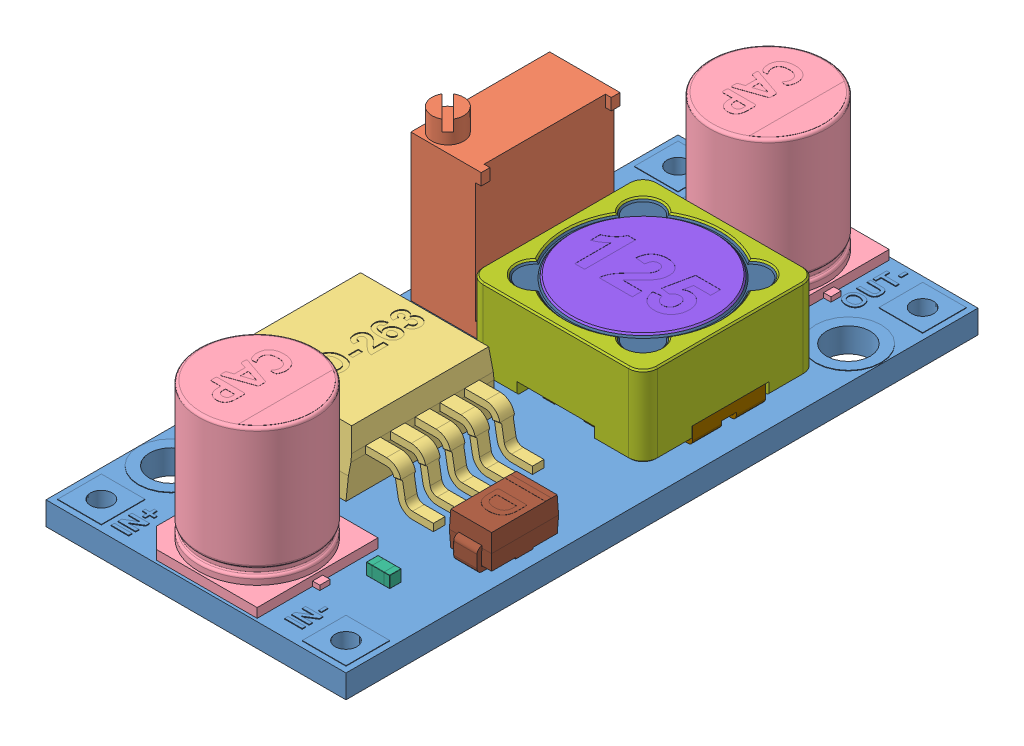
SolidWorks assembly HW-411, configuration По умолчанию. Lengths in mm.
Overall size (20.6 13.97 43.4).
17 component instances, 12 part files, 33 mates.
Components (placement in the parent):
- Board^HW-411-1: Board^HW-411 [По умолчанию] at origin size (20.6 1.69 43.4) (virtual)
- RES_3296W^HW-411-1: RES_3296W^HW-411 [По умолчанию] at (0.685 1.6 -33.9) x (0 0 1) z (-1 0 0) size (9.53 13.97 4.83) (virtual)
- TO-263-5^HW-411-1: TO-263-5^HW-411 [По умолчанию] at (10.65 1.6 -15.2) x (0 0 -1) z (1 0 0) size (10 4.4 14.8) (virtual)
- CAP_SMD_AL_08.0x10.0^HW-411-1: CAP_SMD_AL_08.0x10.0^HW-411 [По умолчанию] at (10.15 1.6 -4.35) x (0 0 1) z (-1 0 0) size (8.3 10.01 9.3) (virtual)
- CAP_SMD_AL_08.0x10.0^HW-411-2: CAP_SMD_AL_08.0x10.0^HW-411 [По умолчанию] at (10.55 1.6 -39.05) x (0 0 1) z (-1 0 0) size (8.3 10.01 9.3) (virtual)
- RES_SMD_0603^HW-411-1: RES_SMD_0603^HW-411 [По умолчанию] at (1 1.6 -22.25) size (1.6 0.39 0.85) (virtual)
- CAP_SMD_0603_H0.50^HW-411-1: CAP_SMD_0603_H0.50^HW-411 [По умолчанию] at (4.6 1.6 -22.3) size (1.6 0.8 0.8) (virtual)
- CAP_SMD_0603_H0.50^HW-411-2: CAP_SMD_0603_H0.50^HW-411 [По умолчанию] at (15.5 2.4 -7.3) x (1 0 0) z (0 0 -1) size (1.6 0.8 0.8) (virtual)
- CDRH125^HW-411-1: CDRH125^HW-411 [По умолчанию] at (13.1 2.1 -27.9) x (0 0 1) z (-1 0 0) size (12 6 12) (virtual)
  - 001^CDRH125_HW-411-1: 001^CDRH125_HW-411 [По умолчанию] at origin size (12 5.5 12) (virtual)
  - 002^CDRH125_HW-411-1: 002^CDRH125_HW-411 [По умолчанию] x (0 0 -1) z (1 0 0) size (10 5.5 10) (virtual)
  - 005^CDRH125_HW-411-1: 005^CDRH125_HW-411 [По умолчанию] at (0 -0.2 0) x (0 0 -1) z (1 0 0) size (4.9 2.22 10.12) (virtual)
  - 005^CDRH125_HW-411-2: 005^CDRH125_HW-411 [По умолчанию] at (0 -0.2 0) x (0 0 1) z (-1 0 0) size (4.9 2.22 10.12) (virtual)
  - 003^CDRH125_HW-411-1: 003^CDRH125_HW-411 [По умолчанию] at (0 4.9 0) size (10.6 0.5 10.6) (virtual)
- Diode_DO214AC(SMA)^HW-411-1: Diode_DO214AC(SMA)^HW-411 [По умолчанию] at (18.45 1.8 -13) x (-1 0 0) z (0 0 -1) size (2.9 2.61 5.3) (virtual)
- LED_0603_Green^HW-411-1: LED_0603_Green^HW-411 [По умолчанию] at (1.6 1.6 -37.6) size (1.6 0.6 0.8) (virtual)
- RES_SMD_0603^HW-411-2: RES_SMD_0603^HW-411 [По умолчанию] at (1.6 1.6 -35.25) size (1.6 0.39 0.85) (virtual)
Mates (geometry in assembly coordinates):
- Концентричный1: concentric anti-aligned: cylinder of RES_3296W^HW-411-1 through (3.1 -0.82 -26.595) axis (0 1 0) radius 0.275; cylinder of Board^HW-411-1 through (3.1 1.6 -26.595) axis (0 -1 0) radius 0.5
- Концентричный2: concentric anti-aligned: cylinder of RES_3296W^HW-411-1 through (3.1 -0.82 -31.675) axis (0 1 0) radius 0.275; cylinder of Board^HW-411-1 through (3.1 1.6 -31.675) axis (0 -1 0) radius 0.5
- Совпадение1: coincident anti-aligned: plane of Board^HW-411-1 through (0 1.6 0) normal (0 1 0); plane of RES_3296W^HW-411-1 through (0.685 1.6 -33.9) normal (0 -1 0)
- Совпадение2: coincident anti-aligned: plane of Board^HW-411-1 through (0 1.6 0) normal (0 1 0); plane of TO-263-5^HW-411-1 through (10.65 1.6 -15.2) normal (0 -1 0)
- Расстояние1: distance = 10.2 mm aligned: plane of TO-263-5^HW-411-1 through (1.4 15.7301 -10.2) normal (0 0 1); plane of Board^HW-411-1 through (0 1.6 0) normal (0 0 1)
- Расстояние2: distance = 1.4 mm: line of TO-263-5^HW-411-1 through (1.4 3.2 -19.45) axis (0 0 1); plane of Board^HW-411-1 through (0 1.6 0) normal (-1 0 0)
- Расстояние3: distance = 0.2 mm aligned: plane of CAP_SMD_AL_08.0x10.0^HW-411-1 through (7.4 2.24 -0.2) normal (0 0 1); plane of Board^HW-411-1 through (0 1.6 0) normal (0 0 1)
- Совпадение6: coincident anti-aligned: plane of Board^HW-411-1 through (0 1.6 0) normal (0 1 0); plane of CAP_SMD_AL_08.0x10.0^HW-411-1 through (10.15 1.6 -4.35) normal (0 -1 0)
- Расстояние4: distance = 6.3 mm aligned: plane of CAP_SMD_AL_08.0x10.0^HW-411-1 through (14.3 2.24 -8.5) normal (1 0 0); plane of Board^HW-411-1 through (20.6 1.6 0) normal (1 0 0)
- Совпадение8: coincident anti-aligned: plane of Board^HW-411-1 through (0 1.6 0) normal (0 1 0); plane of CAP_SMD_AL_08.0x10.0^HW-411-2 through (10.55 1.6 -39.05) normal (0 -1 0)
- Расстояние5: distance = 0.2 mm aligned: plane of Board^HW-411-1 through (0 1.6 -43.4) normal (0 0 -1); plane of CAP_SMD_AL_08.0x10.0^HW-411-2 through (7.8 2.24 -43.2) normal (0 0 -1)
- Расстояние6: distance = 5.9 mm aligned: plane of CAP_SMD_AL_08.0x10.0^HW-411-2 through (14.7 2.24 -43.2) normal (1 0 0); plane of Board^HW-411-1 through (20.6 1.6 0) normal (1 0 0)
- Совпадение11: coincident anti-aligned: plane of Board^HW-411-1 through (0 1.6 0) normal (0 1 0); plane of RES_SMD_0603^HW-411-1 through (2.15 1.6 -22.25) normal (0 -1 0)
- Совпадение12: coincident anti-aligned: plane of Board^HW-411-1 through (0 1.6 0) normal (0 1 0); plane of CAP_SMD_0603_H0.50^HW-411-1 through (5.8 1.6 -22.3) normal (0 -1 0)
- Совпадение181: coincident anti-aligned: plane of Board^HW-411-1 through (0 1.6 0) normal (0 1 0); plane of CAP_SMD_0603_H0.50^HW-411-2 through (16.7 1.6 -6.5) normal (0 -1 0)
- Расстояние10: distance = 3.5 mm aligned: plane of CAP_SMD_0603_H0.50^HW-411-2 through (17.1 2.4 -7.3) normal (1 0 0); plane of Board^HW-411-1 through (20.6 1.6 0) normal (1 0 0)
- Расстояние11: distance = 6.5 mm aligned: plane of CAP_SMD_0603_H0.50^HW-411-2 through (16.7 2.4 -6.5) normal (0 0 1); plane of Board^HW-411-1 through (0 1.6 0) normal (0 0 1)
- Расстояние12: distance = 1.5 mm aligned: plane of Board^HW-411-1 through (20.6 1.6 0) normal (1 0 0); plane of CDRH125^HW-411-1/001^CDRH125_HW-411-1 through (19.1 7.6 -27.9) normal (1 0 0)
- Расстояние13: distance = 9.5 mm aligned: plane of CDRH125^HW-411-1/001^CDRH125_HW-411-1 through (13.1 7.6 -33.9) normal (0 0 -1); plane of Board^HW-411-1 through (0 1.6 -43.4) normal (0 0 -1)
- Совпадение23: coincident anti-aligned: plane of Board^HW-411-1 through (0 1.6 0) normal (0 1 0); plane of CDRH125^HW-411-1/005^CDRH125_HW-411-1 through (8.7804 1.6 -30.4) normal (0 -1 0)
- Совпадение24: coincident anti-aligned: plane of Board^HW-411-1 through (0 1.6 0) normal (0 1 0); plane of Diode_DO214AC(SMA)^HW-411-1 through (17.65 1.6 -15.3) normal (0 -1 0)
- Совпадение183: coincident aligned: plane of RES_SMD_0603^HW-411-1 through (2.15 1.6 -23.1) normal (0 0 -1); plane of CAP_SMD_0603_H0.50^HW-411-1 through (5.8 1.6 -23.1) normal (0 0 -1)
- Расстояние16: distance = 1 mm aligned: plane of RES_SMD_0603^HW-411-1 through (1 1.6 -22.25) normal (-1 0 0); plane of Board^HW-411-1 through (0 1.6 0) normal (-1 0 0)
- Расстояние17: distance = 2 mm anti-aligned: plane of CAP_SMD_0603_H0.50^HW-411-1 through (4.6 1.6 -22.3) normal (-1 0 0); plane of RES_SMD_0603^HW-411-1 through (2.6 1.6 -22.25) normal (1 0 0)
- Расстояние18: distance = 20.3 mm aligned: plane of CAP_SMD_0603_H0.50^HW-411-1 through (5.8 1.6 -23.1) normal (0 0 -1); plane of Board^HW-411-1 through (0 1.6 -43.4) normal (0 0 -1)
- Расстояние20: distance = 10.7 mm: plane of Board^HW-411-1 through (0 1.6 0) normal (0 0 1); line of Diode_DO214AC(SMA)^HW-411-1 through (19.9 3 -10.7) axis (-1 0 0)
- Расстояние21: distance = 0.7 mm: plane of Board^HW-411-1 through (20.6 1.6 0) normal (1 0 0); line of Diode_DO214AC(SMA)^HW-411-1 through (19.9 3 -15.3) axis (0 0 1)
- Совпадение184: coincident anti-aligned: plane of Board^HW-411-1 through (0 1.6 0) normal (0 1 0); plane of LED_0603_Green^HW-411-1 through (3 1.6 -37.6) normal (0 -1 0)
- Расстояние22: distance = 5 mm aligned: plane of Board^HW-411-1 through (0 1.6 -43.4) normal (0 0 -1); plane of LED_0603_Green^HW-411-1 through (3 1.6 -38.4) normal (0 0 -1)
- Расстояние23: distance = 1.6 mm aligned: plane of LED_0603_Green^HW-411-1 through (1.6 1.6 -37.6) normal (-1 0 0); plane of Board^HW-411-1 through (0 1.6 0) normal (-1 0 0)
- Совпадение187: coincident anti-aligned: plane of Board^HW-411-1 through (0 1.6 0) normal (0 1 0); plane of RES_SMD_0603^HW-411-2 through (2.75 1.6 -35.25) normal (0 -1 0)
- Совпадение188: coincident aligned: plane of LED_0603_Green^HW-411-1 through (1.6 1.6 -37.6) normal (-1 0 0); plane of RES_SMD_0603^HW-411-2 through (1.6 1.6 -35.25) normal (-1 0 0)
- Расстояние24: distance = 1.5 mm anti-aligned: plane of LED_0603_Green^HW-411-1 through (3 1.9 -37.6) normal (0 0 1); plane of RES_SMD_0603^HW-411-2 through (2.75 1.6 -36.1) normal (0 0 -1)
